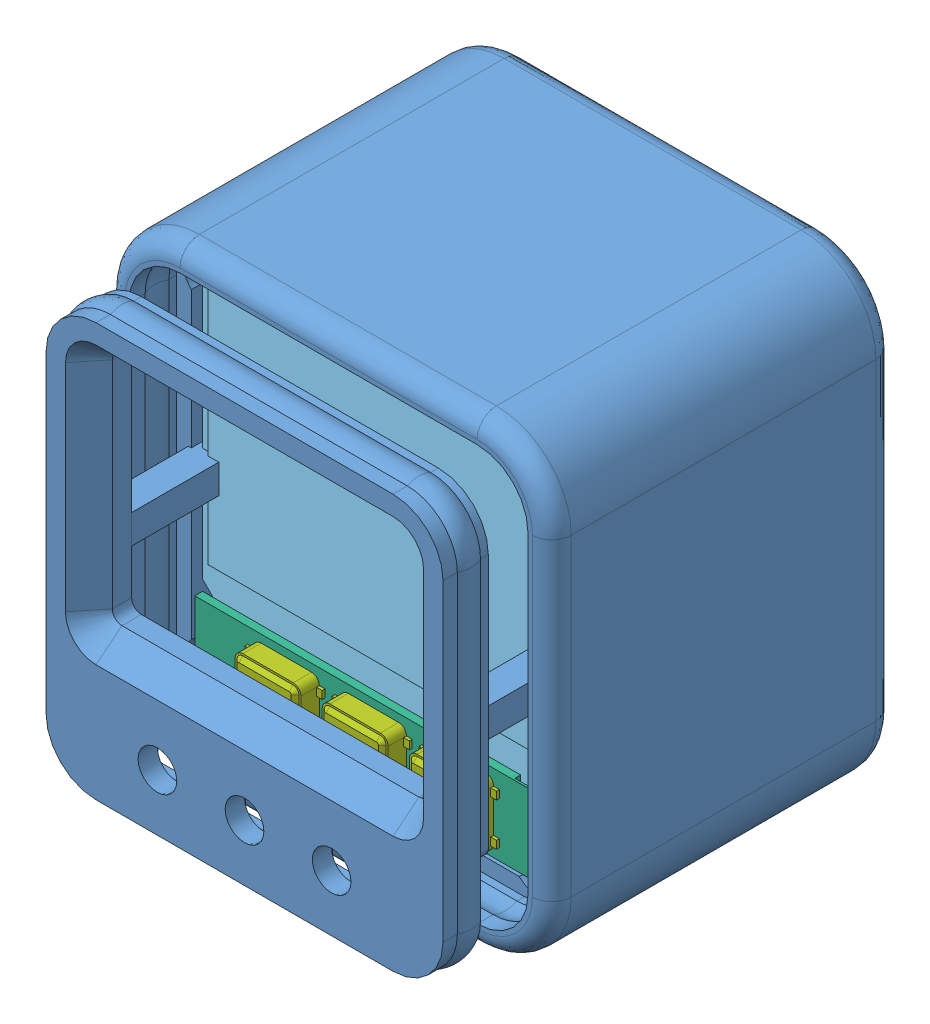
SolidWorks assembly 外壳-方案2-PL_LC打印, configuration 默认. Lengths in mm.
Overall size (23.06 23.9 22.08).
20 component instances, 11 part files, 6 mates.
Components (placement in the parent):
- 外壳-方案2-PL_LC打印_连接零件-1: 外壳-方案2-PL_LC打印_连接零件 [默认] at (-0.3795 -4.3006 1.1613) size (23.06 23.9 22.08)
- 外壳-方案2-盖子_LC打印-1: 外壳-方案2-盖子_LC打印 [默认] at (-0.3795 -4.3006 5.6013) size (20.8 21.64 2.34) (hidden)
- SAU-G0+EX_AHT-PL_PCB-1: SAU-G0+EX_AHT-PL_PCB [默认] at (-8.3432 -18.8134 -16.5369) size (20.36 19.5 16.09)
  - SAU-G0_PCB-1: SAU-G0_PCB [默认] at (11.8444 27.5987 -11.0527) size (20.36 19.5 15.06)
    - SAU-G0_STEP_AD-1: SAU-G0_STEP_AD [默认] at (-16.5787 -13.328 24.4103) size (18.66 19.5 12.19)
    - 2.00mm_2x2_垫板PCB_厚1.0mm-1: 2.00mm_2x2_垫板PCB_厚1.0mm [默认] at (3.1013 6.262 22.4106) x (1 0 0) z (0 -1 0) size (4.5 1 4.5)
    - 2.00mm母座2x2-1: 2.00mm母座2x2 [Default] at (4.1013 6.262 18.1106) x (1 0 0) z (0 1 0) size (4.5 7.1 4.5)
    - 2.00mm_2x2_垫板PCB_厚1.0mm-2: 2.00mm_2x2_垫板PCB_厚1.0mm [默认] at (-10.8587 6.262 22.4106) x (-1 0 0) z (0 1 0) size (4.5 1 4.5)
    - 2.00mm母座2x2-2: 2.00mm母座2x2 [Default] at (-11.8587 6.262 18.1106) x (-1 0 0) z (0 -1 0) size (4.5 7.1 4.5)
    - 0.66寸_64x48_TOP_FPC背面距离背板1mm-1: 0.66寸_64x48_TOP_FPC背面距离背板1mm [Default] at (-3.8787 8.514 25.9703) x (1 0 0) z (0 -1 0) size (18.46 2.27 19.3)
    - 轻触开关+柔性PCB-1: 轻触开关+柔性PCB [默认] at (-0.958 10.42 26.3367) x (1 0 0) z (0 -1 0) size (20.26 5.16 4.01)
      - 方案2-轻触开关_柔性PCB-1: 方案2-轻触开关_柔性PCB [默认] at (-12.1506 0.4339 17.21) size (20.26 3.56 4.01)
      - 轻触开关3x3.5x1.5_3x4.0x2.0-1: 轻触开关3x3.5x1.5_3x4.0x2.0 [默认] at (-2.9206 0.5339 19.31) size (4 1.6 3.4)
      - 轻触开关3x3.5x1.5_3x4.0x2.0-2: 轻触开关3x3.5x1.5_3x4.0x2.0 [默认] at (1.5794 0.5339 19.31) size (4 1.6 3.4)
      - 轻触开关3x3.5x1.5_3x4.0x2.0-3: 轻触开关3x3.5x1.5_3x4.0x2.0 [默认] at (-7.4206 0.5339 19.31) size (4 1.6 3.4)
  - SAU-G0-EX_AHT-PL_PCB-1: SAU-G0-EX_AHT-PL_PCB [默认] at (-1.3662 16.7088 5.0579) x (-1 0 0) z (0 0 -1) size (18.66 19.5 9.43)
    - SAU-G0-EX_AHT-PL_STEP_AD-1: SAU-G0-EX_AHT-PL_STEP_AD [默认] at (23.688 -2.438 0) x (-1 0 0) z (0 0 -1) size (18.66 19.5 3.73)
    - 2.0mm排针2x2-1: 2.0mm排针2x2 [Default] at (-1.352 18.152 0) x (1 0 0) z (0 1 0) size (4 8.2 4)
    - 2.0mm排针2x2-2: 2.0mm排针2x2 [Default] at (-17.312 16.152 0) x (-1 0 0) z (0 -1 0) size (4 8.2 4)
  - 601419(18.5x13.5x6.2mm)_3.7V_100mAh-1: 601419(18.5x13.5x6.2mm)_3.7V_100mAh [Default] at (17.2978 24.8608 6.9079) x (0 -1 0) z (-1 0 0) size (13.5 6.2 18)
Mates (geometry in assembly coordinates):
- 同心1: concentric aligned: cylinder of 外壳-方案2-PL_LC打印_连接零件-1 through (7.2905 -0.4406 -0.8387) axis (0 0 1) radius 2.6304; cylinder of 外壳-方案2-盖子_LC打印-1 through (7.2905 -0.4406 -11.6987) axis (0 0 1) radius 2.5804
- 同心2: concentric aligned: cylinder of 外壳-方案2-PL_LC打印_连接零件-1 through (-8.0495 15.7394 -0.8387) axis (0 0 1) radius 2.6304; cylinder of 外壳-方案2-盖子_LC打印-1 through (-8.0495 15.7394 -11.6987) axis (0 0 1) radius 2.5804
- 距离1: distance = 2 mm anti-aligned: plane of 外壳-方案2-盖子_LC打印-1 through (-0.3795 -4.3006 3.6013) normal (0 0 -1); plane of 外壳-方案2-PL_LC打印_连接零件-1 through (7.2905 15.7394 1.6013) normal (0 0 1)
- 距离2: distance = 2.83 mm anti-aligned: plane of SAU-G0+EX_AHT-PL_PCB-1/SAU-G0-EX_AHT-PL_PCB-1/SAU-G0-EX_AHT-PL_STEP_AD-1 through (-1.112 7.117 -12.4087) normal (0 0 -1); plane of 外壳-方案2-PL_LC打印_连接零件-1 through (-0.3795 -4.3006 -15.2387) normal (0 0 1)
- 距离3: distance = 0.2 mm anti-aligned: plane of SAU-G0+EX_AHT-PL_PCB-1/SAU-G0-EX_AHT-PL_PCB-1/SAU-G0-EX_AHT-PL_STEP_AD-1 through (-9.7095 17.3994 -12.4087) normal (-1 0 0); plane of 外壳-方案2-PL_LC打印_连接零件-1 through (-9.9095 -2.3006 -38.2029) normal (1 0 0)
- 距离4: distance = 0.2 mm anti-aligned: plane of SAU-G0+EX_AHT-PL_PCB-1/SAU-G0_PCB-1/SAU-G0_STEP_AD-1 through (-9.7095 17.3994 -4.179) normal (0 1 0); plane of 外壳-方案2-PL_LC打印_连接零件-1 through (9.1505 17.5994 -38.2029) normal (0 -1 0)
